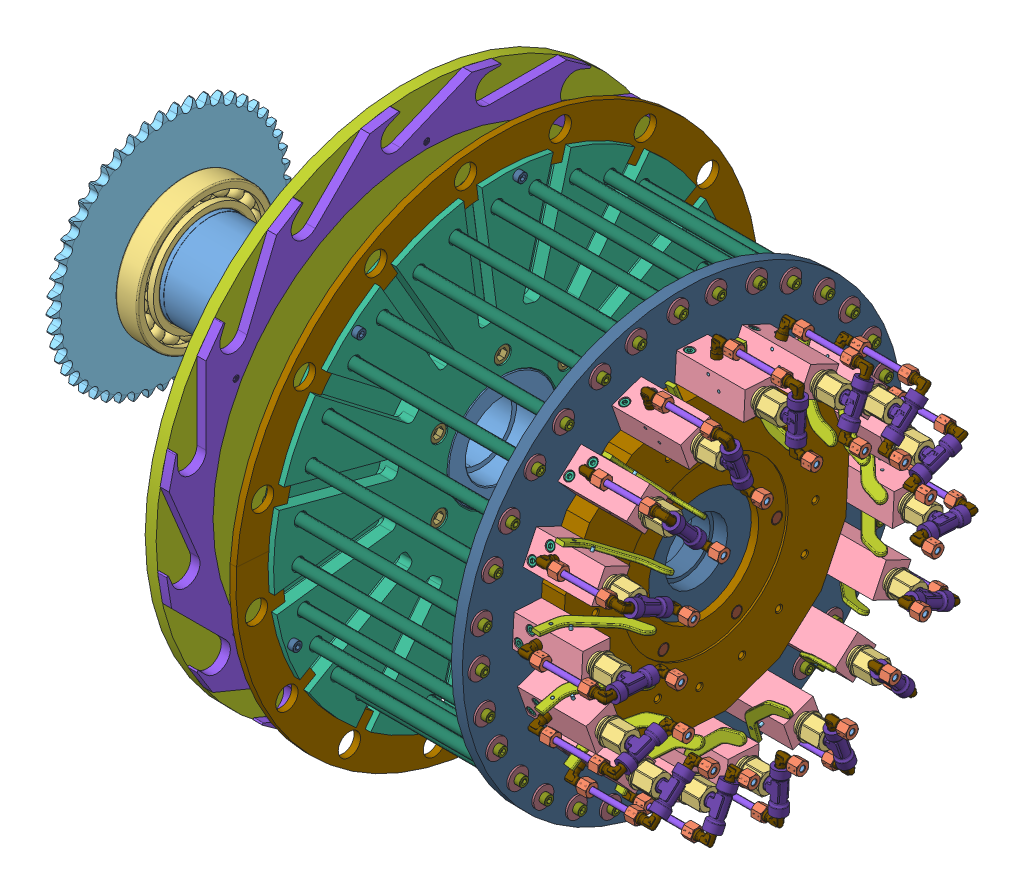
SolidWorks assembly assieme parte rotante, configuration Default. Lengths in mm. (continued)
Components (placement in the parent): (continued)
- AssiemeValvola-7: AssiemeValvola [Default] at (515.3257 -134.8578 488.6421) x (0 0.901303 -0.433189) z (0 -0.433189 -0.901303) size (90.26 138.63 38)
  - RaccordoT-1: RaccordoT [Default] at origin size (43 29.75 16.5)
  - Raccordo a L-1: Raccordo a L [Default] at (-30 0 0) x (0 -1 0) z (0 0 -1) size (28.34 25.51 14.01)
    - 1809_06_10_01-1: 1809_06_10_01 [Default] at origin size (22.49 23 10)
    - 1809_06_10_02-1: 1809_06_10_02 [Default] at origin size (6.5 8.5 8.5)
    - 1809_06_10_03-1: 1809_06_10_03 [Default] at origin size (11.02 15.01 14.01)
  - Raccordo a L-2: Raccordo a L [Default] at (30 0 0) x (0 1 0) z (0 0 -1) size (28.34 25.51 14.01)
    - 1809_06_10_01-1: 1809_06_10_01 [Default] at origin size (22.49 23 10)
    - 1809_06_10_02-1: 1809_06_10_02 [Default] at origin size (6.5 8.5 8.5)
    - 1809_06_10_03-1: 1809_06_10_03 [Default] at origin size (11.02 15.01 14.01)
  - TappoChiusura-1: TappoChiusura [Default] at (0 -32 0) x (0 -1 0) z (0 0 1) size (38.28 26.74 26.74)
  - CorpoValvola-1: CorpoValvola [Default] at (-15 -115.2824 0) size (30 75 34)
  - Raccordo a L-3: Raccordo a L [Default] at (-30 -88.2824 0) x (0 1 0) z (0 0 1) size (28.34 25.51 14.01)
    - 1809_06_10_01-1: 1809_06_10_01 [Default] at origin size (22.49 23 10)
    - 1809_06_10_02-1: 1809_06_10_02 [Default] at origin size (6.5 8.5 8.5)
    - 1809_06_10_03-1: 1809_06_10_03 [Default] at origin size (11.02 15.01 14.01)
  - Spina_3x38-1: Spina_3x38 [Default] at (0 -68.2824 -21) x (-1 0 0) z (0 0 1) size (3 3 38)
  - Spina_3x38-2: Spina_3x38 [Default] at (-10 -80.2824 -21) x (0.996193 0.087174 0) z (0 0 1) size (3 3 38)
  - M5 40mm-3: M5 40mm [ISO 4762 M5 x 40 - 40N] at (-14.6 -108.7824 9) size (45 8.5 8.5)
  - M5 40mm-2: M5 40mm [ISO 4762 M5 x 40 - 40N] at (-14.6 -96.7824 -9) size (45 8.5 8.5)
  - LevaValvola-1: LevaValvola [Default] at (-24.507 -86.571 -17) x (0.996193 0.087174 0) z (0 0 1) size (77.55 60.2 4)
  - Tubo-1: Tubo [Default] at (-30 -15.9665 0) x (1 0 0) z (0 -1 0) size (6 6 56.4)
- AssiemeValvola-8: AssiemeValvola [Default] at (515.3257 -95.0129 541.6718) x (0 0.666921 -0.745128) z (0 -0.745128 -0.666921) size (90.26 138.63 38)
  - RaccordoT-1: RaccordoT [Default] at origin size (43 29.75 16.5)
  - Raccordo a L-1: Raccordo a L [Default] at (-30 0 0) x (0 -1 0) z (0 0 -1) size (28.34 25.51 14.01)
    - 1809_06_10_01-1: 1809_06_10_01 [Default] at origin size (22.49 23 10)
    - 1809_06_10_02-1: 1809_06_10_02 [Default] at origin size (6.5 8.5 8.5)
    - 1809_06_10_03-1: 1809_06_10_03 [Default] at origin size (11.02 15.01 14.01)
  - Raccordo a L-2: Raccordo a L [Default] at (30 0 0) x (0 1 0) z (0 0 -1) size (28.34 25.51 14.01)
    - 1809_06_10_01-1: 1809_06_10_01 [Default] at origin size (22.49 23 10)
    - 1809_06_10_02-1: 1809_06_10_02 [Default] at origin size (6.5 8.5 8.5)
    - 1809_06_10_03-1: 1809_06_10_03 [Default] at origin size (11.02 15.01 14.01)
  - TappoChiusura-1: TappoChiusura [Default] at (0 -32 0) x (0 -1 0) z (0 0 1) size (38.28 26.74 26.74)
  - CorpoValvola-1: CorpoValvola [Default] at (-15 -115.2824 0) size (30 75 34)
  - Raccordo a L-3: Raccordo a L [Default] at (-30 -88.2824 0) x (0 1 0) z (0 0 1) size (28.34 25.51 14.01)
    - 1809_06_10_01-1: 1809_06_10_01 [Default] at origin size (22.49 23 10)
    - 1809_06_10_02-1: 1809_06_10_02 [Default] at origin size (6.5 8.5 8.5)
    - 1809_06_10_03-1: 1809_06_10_03 [Default] at origin size (11.02 15.01 14.01)
  - Spina_3x38-1: Spina_3x38 [Default] at (0 -68.2824 -21) x (-1 0 0) z (0 0 1) size (3 3 38)
  - Spina_3x38-2: Spina_3x38 [Default] at (-10 -80.2824 -21) x (0.996193 0.087174 0) z (0 0 1) size (3 3 38)
  - M5 40mm-3: M5 40mm [ISO 4762 M5 x 40 - 40N] at (-14.6 -108.7824 9) size (45 8.5 8.5)
  - M5 40mm-2: M5 40mm [ISO 4762 M5 x 40 - 40N] at (-14.6 -96.7824 -9) size (45 8.5 8.5)
  - LevaValvola-1: LevaValvola [Default] at (-24.507 -86.571 -17) x (0.996193 0.087174 0) z (0 0 1) size (77.55 60.2 4)
  - Tubo-1: Tubo [Default] at (-30 -15.9665 0) x (1 0 0) z (0 -1 0) size (6 6 56.4)
- AssiemeValvola-9: AssiemeValvola [Default] at (515.3257 -37.9074 575.4168) x (0 0.331007 -0.943628) z (0 -0.943628 -0.331007) size (90.26 138.63 38)
  - RaccordoT-1: RaccordoT [Default] at origin size (43 29.75 16.5)
  - Raccordo a L-1: Raccordo a L [Default] at (-30 0 0) x (0 -1 0) z (0 0 -1) size (28.34 25.51 14.01)
    - 1809_06_10_01-1: 1809_06_10_01 [Default] at origin size (22.49 23 10)
    - 1809_06_10_02-1: 1809_06_10_02 [Default] at origin size (6.5 8.5 8.5)
    - 1809_06_10_03-1: 1809_06_10_03 [Default] at origin size (11.02 15.01 14.01)
  - Raccordo a L-2: Raccordo a L [Default] at (30 0 0) x (0 1 0) z (0 0 -1) size (28.34 25.51 14.01)
    - 1809_06_10_01-1: 1809_06_10_01 [Default] at origin size (22.49 23 10)
    - 1809_06_10_02-1: 1809_06_10_02 [Default] at origin size (6.5 8.5 8.5)
    - 1809_06_10_03-1: 1809_06_10_03 [Default] at origin size (11.02 15.01 14.01)
  - TappoChiusura-1: TappoChiusura [Default] at (0 -32 0) x (0 -1 0) z (0 0 1) size (38.28 26.74 26.74)
  - CorpoValvola-1: CorpoValvola [Default] at (-15 -115.2824 0) size (30 75 34)
  - Raccordo a L-3: Raccordo a L [Default] at (-30 -88.2824 0) x (0 1 0) z (0 0 1) size (28.34 25.51 14.01)
    - 1809_06_10_01-1: 1809_06_10_01 [Default] at origin size (22.49 23 10)
    - 1809_06_10_02-1: 1809_06_10_02 [Default] at origin size (6.5 8.5 8.5)
    - 1809_06_10_03-1: 1809_06_10_03 [Default] at origin size (11.02 15.01 14.01)
  - Spina_3x38-1: Spina_3x38 [Default] at (0 -68.2824 -21) x (-1 0 0) z (0 0 1) size (3 3 38)
  - Spina_3x38-2: Spina_3x38 [Default] at (-10 -80.2824 -21) x (0.996193 0.087174 0) z (0 0 1) size (3 3 38)
  - M5 40mm-3: M5 40mm [ISO 4762 M5 x 40 - 40N] at (-14.6 -108.7824 9) size (45 8.5 8.5)
  - M5 40mm-2: M5 40mm [ISO 4762 M5 x 40 - 40N] at (-14.6 -96.7824 -9) size (45 8.5 8.5)
  - LevaValvola-1: LevaValvola [Default] at (-24.507 -86.571 -17) x (0.996193 0.087174 0) z (0 0 1) size (77.55 60.2 4)
  - Tubo-1: Tubo [Default] at (-30 -15.9665 0) x (1 0 0) z (0 -1 0) size (6 6 56.4)
- AssiemeValvola-10: AssiemeValvola [Default] at (515.3257 27.7648 584.7399) x (0 -0.055301 -0.99847) z (0 -0.99847 0.055301) size (90.26 138.63 38)
  - RaccordoT-1: RaccordoT [Default] at origin size (43 29.75 16.5)
  - Raccordo a L-1: Raccordo a L [Default] at (-30 0 0) x (0 -1 0) z (0 0 -1) size (28.34 25.51 14.01)
    - 1809_06_10_01-1: 1809_06_10_01 [Default] at origin size (22.49 23 10)
    - 1809_06_10_02-1: 1809_06_10_02 [Default] at origin size (6.5 8.5 8.5)
    - 1809_06_10_03-1: 1809_06_10_03 [Default] at origin size (11.02 15.01 14.01)
  - Raccordo a L-2: Raccordo a L [Default] at (30 0 0) x (0 1 0) z (0 0 -1) size (28.34 25.51 14.01)
    - 1809_06_10_01-1: 1809_06_10_01 [Default] at origin size (22.49 23 10)
    - 1809_06_10_02-1: 1809_06_10_02 [Default] at origin size (6.5 8.5 8.5)
    - 1809_06_10_03-1: 1809_06_10_03 [Default] at origin size (11.02 15.01 14.01)
  - TappoChiusura-1: TappoChiusura [Default] at (0 -32 0) x (0 -1 0) z (0 0 1) size (38.28 26.74 26.74)
  - CorpoValvola-1: CorpoValvola [Default] at (-15 -115.2824 0) size (30 75 34)
  - Raccordo a L-3: Raccordo a L [Default] at (-30 -88.2824 0) x (0 1 0) z (0 0 1) size (28.34 25.51 14.01)
    - 1809_06_10_01-1: 1809_06_10_01 [Default] at origin size (22.49 23 10)
    - 1809_06_10_02-1: 1809_06_10_02 [Default] at origin size (6.5 8.5 8.5)
    - 1809_06_10_03-1: 1809_06_10_03 [Default] at origin size (11.02 15.01 14.01)
  - Spina_3x38-1: Spina_3x38 [Default] at (0 -68.2824 -21) x (-1 0 0) z (0 0 1) size (3 3 38)
  - Spina_3x38-2: Spina_3x38 [Default] at (-10 -80.2824 -21) x (0.996193 0.087174 0) z (0 0 1) size (3 3 38)
  - M5 40mm-3: M5 40mm [ISO 4762 M5 x 40 - 40N] at (-14.6 -108.7824 9) size (45 8.5 8.5)
  - M5 40mm-2: M5 40mm [ISO 4762 M5 x 40 - 40N] at (-14.6 -96.7824 -9) size (45 8.5 8.5)
  - LevaValvola-1: LevaValvola [Default] at (-24.507 -86.571 -17) x (0.996193 0.087174 0) z (0 0 1) size (77.55 60.2 4)
  - Tubo-1: Tubo [Default] at (-30 -15.9665 0) x (1 0 0) z (0 -1 0) size (6 6 56.4)
- AssiemeValvola-11: AssiemeValvola [Default] at (515.3257 92.0058 568.2215) x (0 -0.433189 -0.901303) z (0 -0.901303 0.433189) size (90.26 138.63 38)
  - RaccordoT-1: RaccordoT [Default] at origin size (43 29.75 16.5)
  - Raccordo a L-1: Raccordo a L [Default] at (-30 0 0) x (0 -1 0) z (0 0 -1) size (28.34 25.51 14.01)
    - 1809_06_10_01-1: 1809_06_10_01 [Default] at origin size (22.49 23 10)
    - 1809_06_10_02-1: 1809_06_10_02 [Default] at origin size (6.5 8.5 8.5)
    - 1809_06_10_03-1: 1809_06_10_03 [Default] at origin size (11.02 15.01 14.01)
  - Raccordo a L-2: Raccordo a L [Default] at (30 0 0) x (0 1 0) z (0 0 -1) size (28.34 25.51 14.01)
    - 1809_06_10_01-1: 1809_06_10_01 [Default] at origin size (22.49 23 10)
    - 1809_06_10_02-1: 1809_06_10_02 [Default] at origin size (6.5 8.5 8.5)
    - 1809_06_10_03-1: 1809_06_10_03 [Default] at origin size (11.02 15.01 14.01)
  - TappoChiusura-1: TappoChiusura [Default] at (0 -32 0) x (0 -1 0) z (0 0 1) size (38.28 26.74 26.74)
  - CorpoValvola-1: CorpoValvola [Default] at (-15 -115.2824 0) size (30 75 34)
  - Raccordo a L-3: Raccordo a L [Default] at (-30 -88.2824 0) x (0 1 0) z (0 0 1) size (28.34 25.51 14.01)
    - 1809_06_10_01-1: 1809_06_10_01 [Default] at origin size (22.49 23 10)
    - 1809_06_10_02-1: 1809_06_10_02 [Default] at origin size (6.5 8.5 8.5)
    - 1809_06_10_03-1: 1809_06_10_03 [Default] at origin size (11.02 15.01 14.01)
  - Spina_3x38-1: Spina_3x38 [Default] at (0 -68.2824 -21) x (-1 0 0) z (0 0 1) size (3 3 38)
  - Spina_3x38-2: Spina_3x38 [Default] at (-10 -80.2824 -21) x (0.996193 0.087174 0) z (0 0 1) size (3 3 38)
  - M5 40mm-3: M5 40mm [ISO 4762 M5 x 40 - 40N] at (-14.6 -108.7824 9) size (45 8.5 8.5)
  - M5 40mm-2: M5 40mm [ISO 4762 M5 x 40 - 40N] at (-14.6 -96.7824 -9) size (45 8.5 8.5)
  - LevaValvola-1: LevaValvola [Default] at (-24.507 -86.571 -17) x (0.996193 0.087174 0) z (0 0 1) size (77.55 60.2 4)
  - Tubo-1: Tubo [Default] at (-30 -15.9665 0) x (1 0 0) z (0 -1 0) size (6 6 56.4)
- AssiemeValvola-12: AssiemeValvola [Default] at (515.3257 145.0355 528.3766) x (0 -0.745128 -0.666921) z (0 -0.666921 0.745128) size (90.26 138.63 38)
  - RaccordoT-1: RaccordoT [Default] at origin size (43 29.75 16.5)
  - Raccordo a L-1: Raccordo a L [Default] at (-30 0 0) x (0 -1 0) z (0 0 -1) size (28.34 25.51 14.01)
    - 1809_06_10_01-1: 1809_06_10_01 [Default] at origin size (22.49 23 10)
    - 1809_06_10_02-1: 1809_06_10_02 [Default] at origin size (6.5 8.5 8.5)
    - 1809_06_10_03-1: 1809_06_10_03 [Default] at origin size (11.02 15.01 14.01)
  - Raccordo a L-2: Raccordo a L [Default] at (30 0 0) x (0 1 0) z (0 0 -1) size (28.34 25.51 14.01)
    - 1809_06_10_01-1: 1809_06_10_01 [Default] at origin size (22.49 23 10)
    - 1809_06_10_02-1: 1809_06_10_02 [Default] at origin size (6.5 8.5 8.5)
    - 1809_06_10_03-1: 1809_06_10_03 [Default] at origin size (11.02 15.01 14.01)
  - TappoChiusura-1: TappoChiusura [Default] at (0 -32 0) x (0 -1 0) z (0 0 1) size (38.28 26.74 26.74)
  - CorpoValvola-1: CorpoValvola [Default] at (-15 -115.2824 0) size (30 75 34)
  - Raccordo a L-3: Raccordo a L [Default] at (-30 -88.2824 0) x (0 1 0) z (0 0 1) size (28.34 25.51 14.01)
    - 1809_06_10_01-1: 1809_06_10_01 [Default] at origin size (22.49 23 10)
    - 1809_06_10_02-1: 1809_06_10_02 [Default] at origin size (6.5 8.5 8.5)
    - 1809_06_10_03-1: 1809_06_10_03 [Default] at origin size (11.02 15.01 14.01)
  - Spina_3x38-1: Spina_3x38 [Default] at (0 -68.2824 -21) x (-1 0 0) z (0 0 1) size (3 3 38)
  - Spina_3x38-2: Spina_3x38 [Default] at (-10 -80.2824 -21) x (0.996193 0.087174 0) z (0 0 1) size (3 3 38)
  - M5 40mm-3: M5 40mm [ISO 4762 M5 x 40 - 40N] at (-14.6 -108.7824 9) size (45 8.5 8.5)
  - M5 40mm-2: M5 40mm [ISO 4762 M5 x 40 - 40N] at (-14.6 -96.7824 -9) size (45 8.5 8.5)
  - LevaValvola-1: LevaValvola [Default] at (-24.507 -86.571 -17) x (0.996193 0.087174 0) z (0 0 1) size (77.55 60.2 4)
  - Tubo-1: Tubo [Default] at (-30 -15.9665 0) x (1 0 0) z (0 -1 0) size (6 6 56.4)
- AssiemeValvola-13: AssiemeValvola [Default] at (515.3257 178.7805 471.2711) x (0 -0.943628 -0.331007) z (0 -0.331007 0.943628) size (90.26 138.63 38)
  - RaccordoT-1: RaccordoT [Default] at origin size (43 29.75 16.5)
  - Raccordo a L-1: Raccordo a L [Default] at (-30 0 0) x (0 -1 0) z (0 0 -1) size (28.34 25.51 14.01)
    - 1809_06_10_01-1: 1809_06_10_01 [Default] at origin size (22.49 23 10)
    - 1809_06_10_02-1: 1809_06_10_02 [Default] at origin size (6.5 8.5 8.5)
    - 1809_06_10_03-1: 1809_06_10_03 [Default] at origin size (11.02 15.01 14.01)
  - Raccordo a L-2: Raccordo a L [Default] at (30 0 0) x (0 1 0) z (0 0 -1) size (28.34 25.51 14.01)
    - 1809_06_10_01-1: 1809_06_10_01 [Default] at origin size (22.49 23 10)
    - 1809_06_10_02-1: 1809_06_10_02 [Default] at origin size (6.5 8.5 8.5)
    - 1809_06_10_03-1: 1809_06_10_03 [Default] at origin size (11.02 15.01 14.01)
  - TappoChiusura-1: TappoChiusura [Default] at (0 -32 0) x (0 -1 0) z (0 0 1) size (38.28 26.74 26.74)
  - CorpoValvola-1: CorpoValvola [Default] at (-15 -115.2824 0) size (30 75 34)
  - Raccordo a L-3: Raccordo a L [Default] at (-30 -88.2824 0) x (0 1 0) z (0 0 1) size (28.34 25.51 14.01)
    - 1809_06_10_01-1: 1809_06_10_01 [Default] at origin size (22.49 23 10)
    - 1809_06_10_02-1: 1809_06_10_02 [Default] at origin size (6.5 8.5 8.5)
    - 1809_06_10_03-1: 1809_06_10_03 [Default] at origin size (11.02 15.01 14.01)
  - Spina_3x38-1: Spina_3x38 [Default] at (0 -68.2824 -21) x (-1 0 0) z (0 0 1) size (3 3 38)
  - Spina_3x38-2: Spina_3x38 [Default] at (-10 -80.2824 -21) x (0.996193 0.087174 0) z (0 0 1) size (3 3 38)
  - M5 40mm-3: M5 40mm [ISO 4762 M5 x 40 - 40N] at (-14.6 -108.7824 9) size (45 8.5 8.5)
  - M5 40mm-2: M5 40mm [ISO 4762 M5 x 40 - 40N] at (-14.6 -96.7824 -9) size (45 8.5 8.5)
  - LevaValvola-1: LevaValvola [Default] at (-24.507 -86.571 -17) x (0.996193 0.087174 0) z (0 0 1) size (77.55 60.2 4)
  - Tubo-1: Tubo [Default] at (-30 -15.9665 0) x (1 0 0) z (0 -1 0) size (6 6 56.4)
- AssiemeValvola-14: AssiemeValvola [Default] at (515.3257 188.1036 405.5989) x (0 -0.99847 0.055301) z (0 0.055301 0.99847) size (90.26 138.63 38)
  - RaccordoT-1: RaccordoT [Default] at origin size (43 29.75 16.5)
  - Raccordo a L-1: Raccordo a L [Default] at (-30 0 0) x (0 -1 0) z (0 0 -1) size (28.34 25.51 14.01)
    - 1809_06_10_01-1: 1809_06_10_01 [Default] at origin size (22.49 23 10)
    - 1809_06_10_02-1: 1809_06_10_02 [Default] at origin size (6.5 8.5 8.5)
    - 1809_06_10_03-1: 1809_06_10_03 [Default] at origin size (11.02 15.01 14.01)
  - Raccordo a L-2: Raccordo a L [Default] at (30 0 0) x (0 1 0) z (0 0 -1) size (28.34 25.51 14.01)
    - 1809_06_10_01-1: 1809_06_10_01 [Default] at origin size (22.49 23 10)
    - 1809_06_10_02-1: 1809_06_10_02 [Default] at origin size (6.5 8.5 8.5)
    - 1809_06_10_03-1: 1809_06_10_03 [Default] at origin size (11.02 15.01 14.01)
  - TappoChiusura-1: TappoChiusura [Default] at (0 -32 0) x (0 -1 0) z (0 0 1) size (38.28 26.74 26.74)
  - CorpoValvola-1: CorpoValvola [Default] at (-15 -115.2824 0) size (30 75 34)
  - Raccordo a L-3: Raccordo a L [Default] at (-30 -88.2824 0) x (0 1 0) z (0 0 1) size (28.34 25.51 14.01)
    - 1809_06_10_01-1: 1809_06_10_01 [Default] at origin size (22.49 23 10)
    - 1809_06_10_02-1: 1809_06_10_02 [Default] at origin size (6.5 8.5 8.5)
    - 1809_06_10_03-1: 1809_06_10_03 [Default] at origin size (11.02 15.01 14.01)
  - Spina_3x38-1: Spina_3x38 [Default] at (0 -68.2824 -21) x (-1 0 0) z (0 0 1) size (3 3 38)
  - Spina_3x38-2: Spina_3x38 [Default] at (-10 -80.2824 -21) x (0.996193 0.087174 0) z (0 0 1) size (3 3 38)
  - M5 40mm-3: M5 40mm [ISO 4762 M5 x 40 - 40N] at (-14.6 -108.7824 9) size (45 8.5 8.5)
  - M5 40mm-2: M5 40mm [ISO 4762 M5 x 40 - 40N] at (-14.6 -96.7824 -9) size (45 8.5 8.5)
  - LevaValvola-1: LevaValvola [Default] at (-24.507 -86.571 -17) x (0.996193 0.087174 0) z (0 0 1) size (77.55 60.2 4)
  - Tubo-1: Tubo [Default] at (-30 -15.9665 0) x (1 0 0) z (0 -1 0) size (6 6 56.4)
- AssiemeValvola-15: AssiemeValvola [Default] at (515.3257 171.5852 341.3579) x (0 -0.901303 0.433189) z (0 0.433189 0.901303) size (90.26 138.63 38)
  - RaccordoT-1: RaccordoT [Default] at origin size (43 29.75 16.5)
  - Raccordo a L-1: Raccordo a L [Default] at (-30 0 0) x (0 -1 0) z (0 0 -1) size (28.34 25.51 14.01)
    - 1809_06_10_01-1: 1809_06_10_01 [Default] at origin size (22.49 23 10)
    - 1809_06_10_02-1: 1809_06_10_02 [Default] at origin size (6.5 8.5 8.5)
    - 1809_06_10_03-1: 1809_06_10_03 [Default] at origin size (11.02 15.01 14.01)
  - Raccordo a L-2: Raccordo a L [Default] at (30 0 0) x (0 1 0) z (0 0 -1) size (28.34 25.51 14.01)
    - 1809_06_10_01-1: 1809_06_10_01 [Default] at origin size (22.49 23 10)
    - 1809_06_10_02-1: 1809_06_10_02 [Default] at origin size (6.5 8.5 8.5)
    - 1809_06_10_03-1: 1809_06_10_03 [Default] at origin size (11.02 15.01 14.01)
  - TappoChiusura-1: TappoChiusura [Default] at (0 -32 0) x (0 -1 0) z (0 0 1) size (38.28 26.74 26.74)
  - CorpoValvola-1: CorpoValvola [Default] at (-15 -115.2824 0) size (30 75 34)
  - Raccordo a L-3: Raccordo a L [Default] at (-30 -88.2824 0) x (0 1 0) z (0 0 1) size (28.34 25.51 14.01)
    - 1809_06_10_01-1: 1809_06_10_01 [Default] at origin size (22.49 23 10)
    - 1809_06_10_02-1: 1809_06_10_02 [Default] at origin size (6.5 8.5 8.5)
    - 1809_06_10_03-1: 1809_06_10_03 [Default] at origin size (11.02 15.01 14.01)
  - Spina_3x38-1: Spina_3x38 [Default] at (0 -68.2824 -21) x (-1 0 0) z (0 0 1) size (3 3 38)
  - Spina_3x38-2: Spina_3x38 [Default] at (-10 -80.2824 -21) x (0.996193 0.087174 0) z (0 0 1) size (3 3 38)
  - M5 40mm-3: M5 40mm [ISO 4762 M5 x 40 - 40N] at (-14.6 -108.7824 9) size (45 8.5 8.5)
  - M5 40mm-2: M5 40mm [ISO 4762 M5 x 40 - 40N] at (-14.6 -96.7824 -9) size (45 8.5 8.5)
  - LevaValvola-1: LevaValvola [Default] at (-24.507 -86.571 -17) x (0.996193 0.087174 0) z (0 0 1) size (77.55 60.2 4)
  - Tubo-1: Tubo [Default] at (-30 -15.9665 0) x (1 0 0) z (0 -1 0) size (6 6 56.4)
- AssiemeValvola-16: AssiemeValvola [Default] at (515.3257 131.7403 288.3282) x (0 -0.666921 0.745128) z (0 0.745128 0.666921) size (90.26 138.63 38)
  - RaccordoT-1: RaccordoT [Default] at origin size (43 29.75 16.5)
  - Raccordo a L-1: Raccordo a L [Default] at (-30 0 0) x (0 -1 0) z (0 0 -1) size (28.34 25.51 14.01)
    - 1809_06_10_01-1: 1809_06_10_01 [Default] at origin size (22.49 23 10)
    - 1809_06_10_02-1: 1809_06_10_02 [Default] at origin size (6.5 8.5 8.5)
    - 1809_06_10_03-1: 1809_06_10_03 [Default] at origin size (11.02 15.01 14.01)
  - Raccordo a L-2: Raccordo a L [Default] at (30 0 0) x (0 1 0) z (0 0 -1) size (28.34 25.51 14.01)
    - 1809_06_10_01-1: 1809_06_10_01 [Default] at origin size (22.49 23 10)
    - 1809_06_10_02-1: 1809_06_10_02 [Default] at origin size (6.5 8.5 8.5)
    - 1809_06_10_03-1: 1809_06_10_03 [Default] at origin size (11.02 15.01 14.01)
  - TappoChiusura-1: TappoChiusura [Default] at (0 -32 0) x (0 -1 0) z (0 0 1) size (38.28 26.74 26.74)
  - CorpoValvola-1: CorpoValvola [Default] at (-15 -115.2824 0) size (30 75 34)
  - Raccordo a L-3: Raccordo a L [Default] at (-30 -88.2824 0) x (0 1 0) z (0 0 1) size (28.34 25.51 14.01)
    - 1809_06_10_01-1: 1809_06_10_01 [Default] at origin size (22.49 23 10)
    - 1809_06_10_02-1: 1809_06_10_02 [Default] at origin size (6.5 8.5 8.5)
    - 1809_06_10_03-1: 1809_06_10_03 [Default] at origin size (11.02 15.01 14.01)
  - Spina_3x38-1: Spina_3x38 [Default] at (0 -68.2824 -21) x (-1 0 0) z (0 0 1) size (3 3 38)
  - Spina_3x38-2: Spina_3x38 [Default] at (-10 -80.2824 -21) x (0.996193 0.087174 0) z (0 0 1) size (3 3 38)
  - M5 40mm-3: M5 40mm [ISO 4762 M5 x 40 - 40N] at (-14.6 -108.7824 9) size (45 8.5 8.5)
  - M5 40mm-2: M5 40mm [ISO 4762 M5 x 40 - 40N] at (-14.6 -96.7824 -9) size (45 8.5 8.5)
  - LevaValvola-1: LevaValvola [Default] at (-24.507 -86.571 -17) x (0.996193 0.087174 0) z (0 0 1) size (77.55 60.2 4)
  - Tubo-1: Tubo [Default] at (-30 -15.9665 0) x (1 0 0) z (0 -1 0) size (6 6 56.4)
- Disco alimentazione guarnizione fi24.4-1: Disco alimentazione guarnizione fi24.4 [Default] at (198.0433 18.3637 415) x (0 0.065403 0.997859) z (-1 0 0) size (570 285 7.35)
- Disco alimentazione guarnizione fi24.4-2: Disco alimentazione guarnizione fi24.4 [Default] at (198.0433 18.3637 415) x (0 -0.065403 -0.997859) z (-1 0 0) size (570 285 7.35)
- m6 12mm-1: m6 12mm [ISO 4762 M6 x 12 - 12N] at (210.0433 200.6849 574.8914) x (-1 0 0) z (0 0.793353 -0.608761) size (18 10 10)
- m6 12mm-7: m6 12mm [ISO 4762 M6 x 12 - 12N] at (210.0433 260.3445 399.1397) x (-1 0 0) z (0 0.793353 -0.608761) size (18 10 10)
- m6 12mm-8: m6 12mm [ISO 4762 M6 x 12 - 12N] at (210.0433 96.3128 185.3694) x (-1 0 0) z (0 0.793353 -0.608761) size (18 10 10)
- m6 12mm-9: m6 12mm [ISO 4762 M6 x 12 - 12N] at (210.0433 -59.5854 644.6306) x (-1 0 0) z (0 -0.793353 -0.608761) size (18 10 10)
- m6 12mm-10: m6 12mm [ISO 4762 M6 x 12 - 12N] at (210.0433 -223.6171 430.8603) x (-1 0 0) z (0 -0.793353 -0.608761) size (18 10 10)
- m6 12mm-11: m6 12mm [ISO 4762 M6 x 12 - 12N] at (210.0433 -163.9575 255.1086) x (-1 0 0) z (0 0.793353 -0.608761) size (18 10 10)
Mates (geometry in assembly coordinates):
- Concentrico1: concentric anti-aligned: circle of albero rotazione piatti-1; circle of seger 100mm-1
- Coincidente1: coincident anti-aligned: plane of albero rotazione piatti-1 through (-143.4567 18.3637 415) normal (-1 0 0); plane of seger 100mm-1 through (-143.4567 18.3637 415) normal (1 0 0)
- Coincidente2: coincident aligned: plane of albero rotazione piatti-1 through (60.413 18.3637 415) normal (0 1 0); plane of seger 100mm-1 through (-146.4567 18.3637 415) normal (0 1 0)
- Concentrico21: concentric aligned: cylinder of albero rotazione piatti-1 through (60.413 18.3637 415) axis (1 0 0) radius 50; cylinder of SKF - 6020 - 20,DE,NC,20_68-1 through (-152.0942 18.3637 415) axis (1 0 0) radius 50
- Coincidente3: coincident anti-aligned: plane of seger 100mm-1 through (-143.4567 18.3637 415) normal (1 0 0); plane of SKF - 6020 - 20,DE,NC,20_68-1 through (-143.4567 -33.4256 439.9823) normal (-1 0 0)
- Concentrico3: concentric aligned: cylinder of albero rotazione piatti-1 through (60.413 18.3637 415) axis (1 0 0) radius 47.5; cylinder of calettatore d95-1 through (-188.8867 18.3637 415) axis (1 0 0) radius 47.5
- Coincidente7: coincident aligned: plane of albero rotazione piatti-1 through (60.413 18.3637 415) normal (0 1 0); plane of calettatore d95-1 through (-173.8867 18.3637 415) normal (0 1 0)
- Concentrico5: concentric aligned: cylinder of albero rotazione piatti-1 through (60.413 18.3637 415) axis (1 0 0) radius 49.75; cylinder of SKF - 6020 - 20,DE,NC,20_68-2 through (41.4058 18.3637 415) axis (1 0 0) radius 50
- Coincidente8: coincident anti-aligned: plane of albero rotazione piatti-1 through (74.0433 18.3637 415) normal (-1 0 0); plane of SKF - 6020 - 20,DE,NC,20_68-2 through (74.0433 -28.0673 437.2803) normal (1 0 0)
- Concentrico6: concentric aligned: cylinder of albero rotazione piatti-1 through (60.413 18.3637 415) axis (1 0 0) radius 60; cylinder of Disco supporto montaggio e Colonne-1 through (5.3377 18.3637 415) axis (1 0 0) radius 60
- Concentrico7: concentric aligned: cylinder of albero rotazione piatti-1 through (101.3656 98.3637 415) axis (1 0 0) radius 6.25; cylinder of Disco supporto montaggio e Colonne-1 through (204.0433 98.3637 415) axis (1 0 0) radius 9.25
- Coincidente9: coincident anti-aligned: plane of albero rotazione piatti-1 through (175.0433 18.3637 415) normal (1 0 0); plane of Disco supporto montaggio e Colonne-1 through (175.0433 18.3637 415) normal (-1 0 0)
- Concentrico8: concentric anti-aligned: cylinder of albero rotazione piatti-1 through (60.413 18.3637 415) axis (1 0 0) radius 60; cylinder of piatto rotante porta tappi-1 through (111.0433 18.3637 415) axis (-1 0 0) radius 60
- Concentrico9: concentric aligned: circle of albero rotazione piatti-1; circle of piatto rotante porta tappi-1
- Coincidente10: coincident anti-aligned: plane of albero rotazione piatti-1 through (119.0433 18.3637 415) normal (-1 0 0); plane of piatto rotante porta tappi-1 through (119.0433 18.3637 415) normal (1 0 0)
- Concentrico10: concentric aligned: cylinder of piatto rotante porta tappi-1 through (119.0433 18.3637 415) axis (-1 0 0) radius 233; cylinder of disco trasportatore tappi 31-1 through (121.0433 18.3637 415) axis (-1 0 0) radius 233
- Tangente2: tangent: cylinder of piatto rotante porta tappi-1 through (98.5243 -101.6363 622.8461) axis (1 0 0) radius 3.25; curve of disco trasportatore tappi 31-1
- Coincidente13: coincident anti-aligned: plane of piatto rotante porta tappi-1 through (111.0433 18.3637 415) normal (1 0 0); plane of disco trasportatore tappi 31-1 through (111.0433 18.3637 415) normal (-1 0 0)
- Concentrico11: concentric anti-aligned: cylinder of albero rotazione piatti-1 through (60.413 18.3637 415) axis (1 0 0) radius 40; cylinder of disco trascinato porta distributore vuoto-1 through (400.0433 18.3637 415) axis (-1 0 0) radius 30
- Concentrico12: concentric anti-aligned: cylinder of Disco supporto montaggio e Colonne-1 through (204.0433 -202.0247 450.2415) axis (1 0 0) radius 6; cylinder of disco trascinato porta distributore vuoto-1 through (417.0139 -202.0247 450.2415) axis (-1 0 0) radius 6
- Coincidente14: coincident anti-aligned: plane of Distributore Rotante-1 through (400.0433 18.3637 415) normal (-1 0 0); plane of disco trascinato porta distributore vuoto-1 through (400.0433 18.3637 415) normal (1 0 0)
- Concentrico13: concentric anti-aligned: circle of Distributore Rotante-1; circle of disco trascinato porta distributore vuoto-1
- Concentrico14: concentric anti-aligned: cylinder of Distributore Rotante-1 through (230.3377 18.3637 415) axis (1 0 0) radius 60; cylinder of disco trascinato porta distributore vuoto-1 through (415.0433 18.3637 415) axis (-1 0 0) radius 67.5
- Concentrico15: concentric anti-aligned: cylinder of disco trascinato porta distributore vuoto-1 through (388.0433 -53.0243 378.8925) axis (1 0 0) radius 6.25; cylinder of m12 35mm-1 through (344.2933 -53.0243 378.8925) axis (-1 0 0) radius 6
- Coincidente15: coincident anti-aligned: plane of disco trascinato porta distributore vuoto-1 through (388.0433 18.3637 415) normal (-1 0 0); plane of m12 35mm-1 through (388.0433 -45.2301 383.3925) normal (1 0 0)
- Parallelo1: parallel anti-aligned: plane of m12 35mm-1 through (382.0433 -47.9668 381.8125) normal (0 -1 0)
- Concentrico16: concentric aligned: cylinder of Disco supporto montaggio e Colonne-1 through (204.0433 -21.6363 345.718) axis (1 0 0) radius 9.25; cylinder of m12 90mm-3 through (234.7933 -21.6363 345.718) axis (1 0 0) radius 6
- Coincidente17: coincident anti-aligned: plane of Disco supporto montaggio e Colonne-1 through (191.0433 -27.049 342.593) normal (1 0 0); plane of m12 90mm-3 through (191.0433 -29.4305 341.218) normal (-1 0 0)
- Parallelo2: parallel aligned: plane of m12 35mm-1 through (382.0433 -47.9668 381.8125) normal (0 -1 0); plane of m12 90mm-3 through (197.0433 -16.5788 348.6379) normal (0 -1 0)
- Concentrico171: concentric anti-aligned: cylinder of piatto rotante porta tappi-1 through (98.5243 -101.6363 207.1539) axis (1 0 0) radius 3.25; cylinder of rondella m6 22mm-1 through (64.1183 -101.6363 207.1539) axis (-1 0 0) radius 3.3
- Coincidente191: coincident anti-aligned: plane of piatto rotante porta tappi-1 through (99.0433 18.3637 415) normal (-1 0 0); plane of rondella m6 22mm-1 through (99.0433 -101.6363 210.4539) normal (1 0 0)
- Parallelo3: parallel anti-aligned: plane of rondella m6 22mm-1 through (99.0433 -101.6363 207.1539) normal (0 -1 0)
- Concentrico181: concentric aligned: cylinder of rondella m6 22mm-1 through (64.1183 -101.6363 207.1539) axis (-1 0 0) radius 3.3; cylinder of M6 20mm-1 through (59.2933 -101.6363 207.1539) axis (-1 0 0) radius 5
- Coincidente211: coincident anti-aligned: plane of rondella m6 22mm-1 through (97.0433 -101.6363 218.1539) normal (-1 0 0); plane of M6 20mm-1 through (97.0433 -97.3062 204.6539) normal (1 0 0)
- Parallelo4: parallel aligned: plane of m12 35mm-1 through (382.0433 -47.9668 381.8125) normal (0 -0.5 -0.866025); plane of M6 20mm-1 through (94.0433 -101.6363 210.0892) normal (0 -0.5 -0.866025)
- Concentrico19: concentric anti-aligned: cylinder of Disco supporto montaggio e Colonne-1 through (204.0433 70.1437 197.9013) axis (1 0 0) radius 6; cylinder of asta scorrimento carello-1 through (400.0433 70.1437 197.9013) axis (-1 0 0) radius 6
- Concentrico201: concentric aligned: cylinder of asta scorrimento carello-1 through (175.0433 70.1437 197.9013) axis (-1 0 0) radius 3.2; cylinder of rondella m6 22mm-7 through (140.1183 70.1437 197.9013) axis (-1 0 0) radius 3.3
- Coincidente231: coincident anti-aligned: plane of asta scorrimento carello-1 through (175.0433 70.1437 197.9013) normal (-1 0 0); plane of rondella m6 22mm-7 through (175.0433 70.1437 201.2013) normal (1 0 0)
- Concentrico211: concentric aligned: cylinder of rondella m6 22mm-7 through (140.1183 70.1437 197.9013) axis (-1 0 0) radius 3.3; cylinder of M6 16mm-1 through (135.2933 70.1437 197.9013) axis (-1 0 0) radius 5
- Coincidente241: coincident anti-aligned: plane of rondella m6 22mm-7 through (173.0433 70.1437 208.9013) normal (-1 0 0); plane of M6 16mm-1 through (173.0433 75.1437 197.9013) normal (1 0 0)
- Parallelo5: parallel aligned: plane of asta scorrimento carello-1 through (287.5433 70.1437 197.9013) normal (0 0 -1); plane of M6 16mm-1 through (170.0433 68.6761 200.4433) normal (0 0 -1)
- Parallelo9: parallel anti-aligned: plane of rondella m6 22mm-7 through (175.0433 70.1437 197.9013) normal (0 0 1); plane of M6 16mm-1 through (170.0433 68.6761 200.4433) normal (0 0 -1)
- Coincidente30: coincident anti-aligned: plane of Disco supporto montaggio e Colonne-1 through (175.0433 18.3637 415) normal (-1 0 0); plane of rondella m6 22mm-7 through (175.0433 70.1437 201.2013) normal (1 0 0)
- Coincidente31: coincident anti-aligned: plane of disco trascinato porta distributore vuoto-1 through (400.0433 18.3637 415) normal (1 0 0); plane of rondella m6 22mm-8 through (400.0433 70.1437 201.2013) normal (-1 0 0)
- Coincidente32: coincident anti-aligned: plane of Distributore Rotante-1 through (400.0433 40.5763 258.5322) normal (0 0.331007 -0.943628); plane of AssiemeValvola-1/CorpoValvola-1 through (400.0433 85.7114 274.3647) normal (0 -0.331007 0.943628)
- Coincidente33: coincident anti-aligned: plane of disco trascinato porta distributore vuoto-1 through (400.0433 18.3637 415) normal (1 0 0); plane of AssiemeValvola-1/CorpoValvola-1 through (400.0433 95.6416 246.0559) normal (-1 0 0)
- Concentrico22: concentric anti-aligned: cylinder of Distributore Rotante-1 through (412.5433 55.4365 309.3136) axis (0 0.331007 -0.943628) radius 3; cylinder of AssiemeValvola-1/CorpoValvola-1 through (412.5433 69.6697 268.7376) axis (0 -0.331007 0.943628) radius 3
- Concentrico23: concentric anti-aligned: cylinder of Disco supporto montaggio e Colonne-1 through (198.0433 18.3637 415) axis (-1 0 0) radius 235; cylinder of Disco alimentazione guarnizione fi24.4-2 through (191.0433 18.3637 415) axis (1 0 0) radius 235
- Concentrico24: concentric anti-aligned: cylinder of Disco supporto montaggio e Colonne-1 through (198.0433 18.3637 415) axis (-1 0 0) radius 235; cylinder of Disco alimentazione guarnizione fi24.4-1 through (191.0433 18.3637 415) axis (1 0 0) radius 235
- Coincidente34: coincident anti-aligned: plane of Disco alimentazione guarnizione fi24.4-1 through (191.0433 33.7334 649.4968) normal (0 -0.997859 0.065403); plane of Disco alimentazione guarnizione fi24.4-2 through (191.0433 37.0036 699.3898) normal (0 0.997859 -0.065403)
- Coincidente35: coincident aligned: plane of Disco alimentazione guarnizione fi24.4-1 through (198.0433 18.3637 415) normal (1 0 0); plane of Disco alimentazione guarnizione fi24.4-2 through (198.0433 18.3637 415) normal (1 0 0)
- Concentrico25: concentric anti-aligned: cylinder of Disco supporto montaggio e Colonne-1 through (188.8509 -59.5854 644.6306) axis (1 0 0) radius 3.25; circle of Disco alimentazione guarnizione fi24.4-2
- Coincidente36: coincident anti-aligned: plane of Disco supporto montaggio e Colonne-1 through (198.0433 18.3637 415) normal (-1 0 0); plane of Disco alimentazione guarnizione fi24.4-2 through (198.0433 18.3637 415) normal (1 0 0)
- Concentrico26: concentric anti-aligned: cylinder of Disco supporto montaggio e Colonne-1 through (188.8509 200.6849 574.8914) axis (1 0 0) radius 3.25; cylinder of M6 16mm-65 through (198.0564 200.6849 574.8914) axis (-1 0 0) radius 3
- Concentrico271: concentric anti-aligned: cone of Disco supporto montaggio e Colonne-1 through (203.0433 200.6849 574.8914) axis (-1 0 0); cylinder of m6 12mm-1 through (241.7933 200.6849 574.8914) axis (1 0 0) radius 5
- Coincidente381: coincident anti-aligned: plane of Disco supporto montaggio e Colonne-1 through (204.0433 18.3637 415) normal (1 0 0); plane of m6 12mm-1 through (204.0433 203.7287 578.8581) normal (-1 0 0)
- Concentrico281: concentric anti-aligned: cone of Disco supporto montaggio e Colonne-1 through (203.0433 260.3445 399.1397) axis (-1 0 0); cylinder of m6 12mm-7 through (241.7933 260.3445 399.1397) axis (1 0 0) radius 5
- Coincidente401: coincident anti-aligned: plane of Disco supporto montaggio e Colonne-1 through (204.0433 18.3637 415) normal (1 0 0); plane of m6 12mm-7 through (204.0433 263.3883 403.1065) normal (-1 0 0)
- Parallelo11: parallel aligned: plane of m6 12mm-1 through (207.0433 198.898 572.5627) normal (0 0.92388 0.382683); plane of m6 12mm-7 through (207.0433 258.5576 396.8111) normal (0 0.92388 0.382683)
- Concentrico291: concentric anti-aligned: cone of Disco supporto montaggio e Colonne-1 through (203.0433 96.3128 185.3694) axis (-1 0 0); cylinder of m6 12mm-8 through (241.7933 96.3128 185.3694) axis (1 0 0) radius 5
- Coincidente421: coincident anti-aligned: plane of Disco supporto montaggio e Colonne-1 through (204.0433 18.3637 415) normal (1 0 0); plane of m6 12mm-8 through (204.0433 99.3566 189.3362) normal (-1 0 0)
- Coincidente44: coincident aligned: plane of m6 12mm-7 through (207.0433 259.2212 401.8516) normal (0 0.793353 -0.608761); plane of m6 12mm-8 through (207.0433 95.1895 188.0813) normal (0 0.793353 -0.608761)
- Concentrico301: concentric anti-aligned: cone of Disco supporto montaggio e Colonne-1 through (203.0433 -59.5854 644.6306) axis (-1 0 0); cylinder of m6 12mm-9 through (241.7933 -59.5854 644.6306) axis (1 0 0) radius 5
- Coincidente451: coincident anti-aligned: plane of Disco supporto montaggio e Colonne-1 through (204.0433 18.3637 415) normal (1 0 0); plane of m6 12mm-9 through (204.0433 -56.5416 640.6638) normal (-1 0 0)
- Concentrico311: concentric anti-aligned: cone of Disco supporto montaggio e Colonne-1 through (203.0433 -223.6171 430.8603) axis (-1 0 0); cylinder of m6 12mm-10 through (241.7933 -223.6171 430.8603) axis (1 0 0) radius 5
- Coincidente461: coincident anti-aligned: plane of Disco supporto montaggio e Colonne-1 through (204.0433 18.3637 415) normal (1 0 0); plane of m6 12mm-10 through (204.0433 -220.5733 426.8935) normal (-1 0 0)
- Concentrico321: concentric anti-aligned: cone of Disco supporto montaggio e Colonne-1 through (203.0433 -163.9575 255.1086) axis (-1 0 0); cylinder of m6 12mm-11 through (241.7933 -163.9575 255.1086) axis (1 0 0) radius 5
- Coincidente471: coincident anti-aligned: plane of Disco supporto montaggio e Colonne-1 through (204.0433 18.3637 415) normal (1 0 0); plane of m6 12mm-11 through (204.0433 -160.9136 259.0754) normal (-1 0 0)
- Parallelo13: parallel aligned: plane of m6 12mm-9 through (207.0433 -62.4955 644.2474) normal (0 0.92388 -0.382683); plane of m6 12mm-10 through (207.0433 -226.5272 430.4771) normal (0 0.92388 -0.382683)
- Parallelo14: parallel aligned: plane of Disco supporto montaggio e Colonne-1 through (191.0433 26.2972 408.9124) normal (0 -0.793353 0.608761); plane of m6 12mm-11 through (207.0433 -162.8342 252.3968) normal (0 -0.793353 0.608761)
- Parallelo15: parallel aligned: plane of Disco supporto montaggio e Colonne-1 through (191.0433 19.669 405.0856) normal (0 -0.130526 0.991445); plane of m6 12mm-10 through (207.0433 -221.8302 428.5316) normal (0 -0.130526 0.991445)
- Concentrico322: concentric anti-aligned: cylinder of albero rotazione piatti-1 through (60.413 18.3637 415) axis (1 0 0) radius 47.5; cylinder of Chain wheel ISO - 50Z 10A-1-1 through (-139.8862 18.3637 415) axis (-1 0 0) radius 47.5
- Coincidente472: coincident anti-aligned: plane of albero rotazione piatti-1 through (-155.9567 18.3637 415) normal (-1 0 0); plane of Chain wheel ISO - 50Z 10A-1-1 through (-155.9567 18.3637 415) normal (1 0 0)
- Parallelo16: parallel aligned: plane of Chain wheel ISO - 50Z 10A-1-1 through (-164.8867 18.3637 415) normal (0 1 0)
- Parallelo17: parallel aligned: plane of calettatore d95-1 through (-173.8867 18.3637 415) normal (0 1 0)
- Coincidente473: coincident anti-aligned: plane of calettatore d95-1 through (-159.8867 84.9137 415) normal (1 0 0); plane of Chain wheel ISO - 50Z 10A-1-1 through (-159.8867 18.3637 415) normal (-1 0 0)
